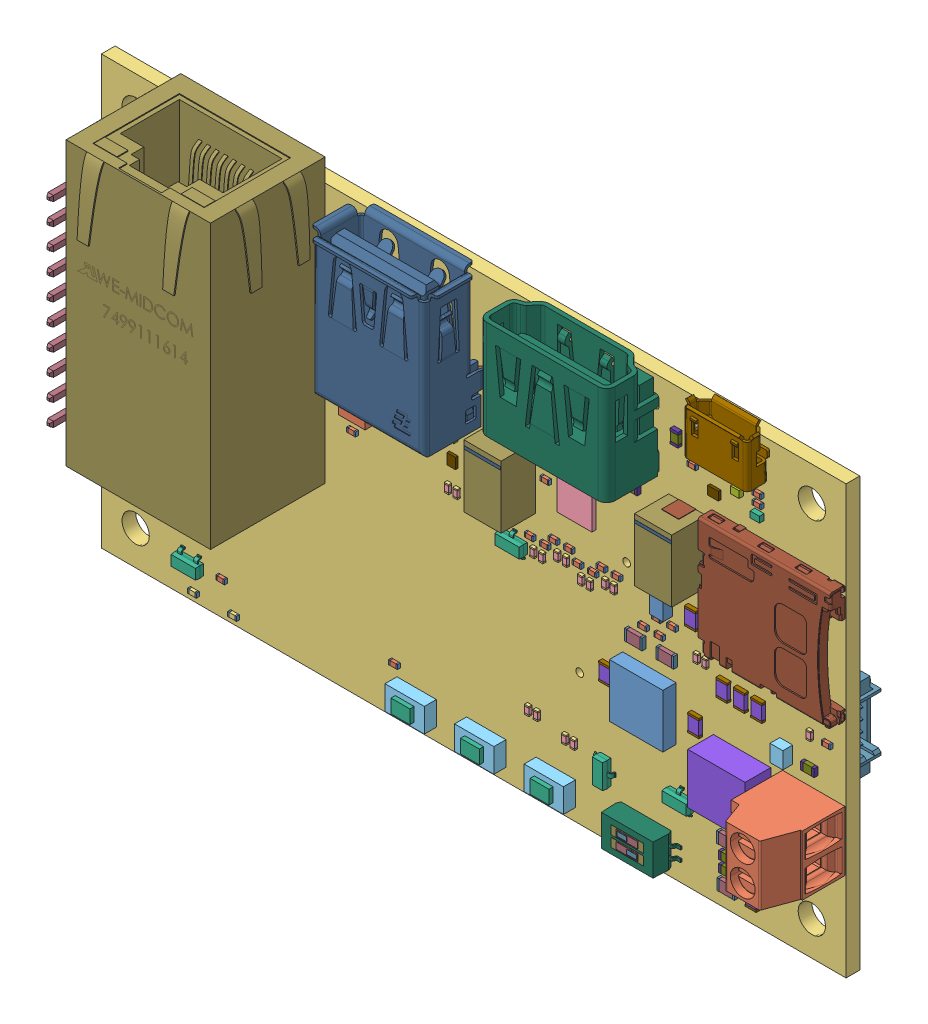
SolidWorks assembly ASG003_3D_MODEL, configuration Default. Lengths in mm. (continued)
Components (placement in the parent): (continued)
- ASG003_3D_MODEL.step-1: ASG003_3D_MODEL.step [Default] at origin size (87.04 52.68 23.65) (continued)
  - D6.step-1: D6.step [Default] at origin size (1 0.8 0.5) (continued)
    - 870940960.step-1: 870940960.step [Default] at (41.166 32.031 0) size (1 0.8 0.5) (continued)
      - Extruded-31.step-1: Extruded-31.step [Default] at origin size (1 0.8 0.5)
  - D5.step-1: D5.step [Default] at origin size (1 0.8 0.5)
    - 870940960.step-1: 870940960.step [Default] at (35.166 32.031 0) size (1 0.8 0.5)
      - Extruded-31.step-1: Extruded-31.step [Default] at origin size (1 0.8 0.5)
  - D4.step-1: D4.step [Default] at origin size (1 0.8 0.5)
    - 870940960.step-1: 870940960.step [Default] at (44.881 32.031 0) size (1 0.8 0.5)
      - Extruded-31.step-1: Extruded-31.step [Default] at origin size (1 0.8 0.5)
  - D2.step-1: D2.step [Default] at origin size (1.02 0.52 0.36)
    - 870944640.step-1: 870944640.step [Default] at (10.9212 1.0646 0) size (1.01 0.51 0.36)
      - Extruded-28.step-1: Extruded-28.step [Default] at origin size (1.01 0.51 0.36)
    - 870940480.step-1: 870940480.step [Default] at (10.4912 1.0646 0) size (0.16 0.52 0.35)
      - Extruded.step-1: Extruded.step [Default] at origin size (0.16 0.52 0.35)
    - 870940480.step-2: 870940480.step [Default] at (11.3512 1.0646 0) size (0.16 0.52 0.35)
      - Extruded.step-1: Extruded.step [Default] at origin size (0.16 0.52 0.35)
  - C57.step-1: C57.step [Default] at origin size (1.3 2.04 0.45)
    - 740904480.step-1: 740904480.step [Default] at (69.215 27.686 0) size (1.25 2 0.45)
      - Extruded-32.step-1: Extruded-32.step [Default] at origin size (1.25 2 0.45)
    - 740902240.step-1: 740902240.step [Default] at (69.215 26.7735 0) size (1.3 0.23 0.45)
      - Extruded-33.step-1: Extruded-33.step [Default] at origin size (1.3 0.23 0.45)
    - 740902240.step-2: 740902240.step [Default] at (69.215 28.586 0) size (1.3 0.23 0.45)
      - Extruded-33.step-1: Extruded-33.step [Default] at origin size (1.3 0.23 0.45)
  - C47.step-1: C47.step [Default] at origin size (1.3 2.04 0.45)
    - 740902240.step-1: 740902240.step [Default] at (72.8972 21.3736 0) size (1.3 0.23 0.45)
      - Extruded-33.step-1: Extruded-33.step [Default] at origin size (1.3 0.23 0.45)
    - 740902240.step-2: 740902240.step [Default] at (72.8972 23.1861 0) size (1.3 0.23 0.45)
      - Extruded-33.step-1: Extruded-33.step [Default] at origin size (1.3 0.23 0.45)
    - 740904480.step-1: 740904480.step [Default] at (72.8972 22.2736 0) size (1.25 2 0.45)
      - Extruded-32.step-1: Extruded-32.step [Default] at origin size (1.25 2 0.45)
  - C46.step-1: C46.step [Default] at origin size (1.3 2.04 0.45)
    - 740902240.step-1: 740902240.step [Default] at (76.9612 21.3736 0) size (1.3 0.23 0.45)
      - Extruded-33.step-1: Extruded-33.step [Default] at origin size (1.3 0.23 0.45)
    - 740902240.step-2: 740902240.step [Default] at (76.9612 23.1861 0) size (1.3 0.23 0.45)
      - Extruded-33.step-1: Extruded-33.step [Default] at origin size (1.3 0.23 0.45)
    - 740904480.step-1: 740904480.step [Default] at (76.9612 22.2736 0) size (1.25 2 0.45)
      - Extruded-32.step-1: Extruded-32.step [Default] at origin size (1.25 2 0.45)
  - C45.step-1: C45.step [Default] at origin size (1.3 2.04 0.45)
    - 740902240.step-1: 740902240.step [Default] at (74.9292 21.3736 0) size (1.3 0.23 0.45)
      - Extruded-33.step-1: Extruded-33.step [Default] at origin size (1.3 0.23 0.45)
    - 740902240.step-2: 740902240.step [Default] at (74.9292 23.1861 0) size (1.3 0.23 0.45)
      - Extruded-33.step-1: Extruded-33.step [Default] at origin size (1.3 0.23 0.45)
    - 740904480.step-1: 740904480.step [Default] at (74.9292 22.2736 0) size (1.25 2 0.45)
      - Extruded-32.step-1: Extruded-32.step [Default] at origin size (1.25 2 0.45)
  - C44.step-1: C44.step [Default] at origin size (1.02 0.52 0.36)
    - 870940480.step-1: 870940480.step [Default] at (29.084 26.6678 0) size (0.16 0.52 0.35)
      - Extruded.step-1: Extruded.step [Default] at origin size (0.16 0.52 0.35)
    - 870940480.step-2: 870940480.step [Default] at (29.944 26.6678 0) size (0.16 0.52 0.35)
      - Extruded.step-1: Extruded.step [Default] at origin size (0.16 0.52 0.35)
    - 870940640.step-1: 870940640.step [Default] at (29.514 26.6678 0) size (1.01 0.51 0.36)
      - Extruded-0.step-1: Extruded-0.step [Default] at origin size (1.01 0.51 0.36)
  - C43.step-1: C43.step [Default] at origin size (1.02 0.52 0.36)
    - 870940480.step-1: 870940480.step [Default] at (76.455 43 0) size (0.16 0.52 0.35)
      - Extruded.step-1: Extruded.step [Default] at origin size (0.16 0.52 0.35)
    - 870940480.step-2: 870940480.step [Default] at (77.315 43 0) size (0.16 0.52 0.35)
      - Extruded.step-1: Extruded.step [Default] at origin size (0.16 0.52 0.35)
    - 870940640.step-1: 870940640.step [Default] at (76.885 43 0) size (1.01 0.51 0.36)
      - Extruded-0.step-1: Extruded-0.step [Default] at origin size (1.01 0.51 0.36)
  - C42.step-1: C42.step [Default] at origin size (1.02 0.52 0.36)
    - 870940480.step-1: 870940480.step [Default] at (76.455 44.016 0) size (0.16 0.52 0.35)
      - Extruded.step-1: Extruded.step [Default] at origin size (0.16 0.52 0.35)
    - 870940480.step-2: 870940480.step [Default] at (77.315 44.016 0) size (0.16 0.52 0.35)
      - Extruded.step-1: Extruded.step [Default] at origin size (0.16 0.52 0.35)
    - 870940640.step-1: 870940640.step [Default] at (76.885 44.016 0) size (1.01 0.51 0.36)
      - Extruded-0.step-1: Extruded-0.step [Default] at origin size (1.01 0.51 0.36)
  - C41.step-1: C41.step [Default] at origin size (1.02 0.52 0.36)
    - 870940480.step-1: 870940480.step [Default] at (68.835 44.143 0) size (0.16 0.52 0.35)
      - Extruded.step-1: Extruded.step [Default] at origin size (0.16 0.52 0.35)
    - 870940480.step-2: 870940480.step [Default] at (69.695 44.143 0) size (0.16 0.52 0.35)
      - Extruded.step-1: Extruded.step [Default] at origin size (0.16 0.52 0.35)
    - 870940640.step-1: 870940640.step [Default] at (69.265 44.143 0) size (1.01 0.51 0.36)
      - Extruded-0.step-1: Extruded-0.step [Default] at origin size (1.01 0.51 0.36)
  - C40.step-1: C40.step [Default] at origin size (4.35 7.4 4.01)
    - 870941440.step-1: 870941440.step [Default] at (68.4522 37.8735 0) size (4.3 0.35 4.01)
      - Extruded-34.step-1: Extruded-34.step [Default] at origin size (4.3 0.35 4.01)
    - 870941600.step-1: 870941600.step [Default] at (68.4522 31.3736 0) size (2 0.2 2)
      - Extruded-35.step-1: Extruded-35.step [Default] at origin size (2 0.2 2)
    - 870941600.step-2: 870941600.step [Default] at (68.4522 38.5736 0) size (2 0.2 2)
      - Extruded-35.step-1: Extruded-35.step [Default] at origin size (2 0.2 2)
    - 870941760.step-1: 870941760.step [Default] at (68.4523 34.9735 0) size (4.35 7.3 4)
      - Extruded-36.step-1: Extruded-36.step [Default] at origin size (4.35 7.3 4)
  - C39.step-1: C39.step [Default] at origin size (1.02 0.52 0.36)
    - 870940480.step-1: 870940480.step [Default] at (39.673 40.1066 -1.9516) size (0.16 0.52 0.35)
      - Extruded.step-1: Extruded.step [Default] at origin size (0.16 0.52 0.35)
    - 870940480.step-2: 870940480.step [Default] at (38.813 40.1066 -1.9516) size (0.16 0.52 0.35)
      - Extruded.step-1: Extruded.step [Default] at origin size (0.16 0.52 0.35)
    - 870940640.step-1: 870940640.step [Default] at (39.243 40.1066 -1.9506) size (1.01 0.51 0.36)
      - Extruded-0.step-1: Extruded-0.step [Default] at origin size (1.01 0.51 0.36)
  - C38.step-1: C38.step [Default] at origin size (1.02 0.52 0.36)
    - 870940480.step-1: 870940480.step [Default] at (49.023 38.174 0) size (0.16 0.52 0.35)
      - Extruded.step-1: Extruded.step [Default] at origin size (0.16 0.52 0.35)
    - 870940480.step-2: 870940480.step [Default] at (49.883 38.174 0) size (0.16 0.52 0.35)
      - Extruded.step-1: Extruded.step [Default] at origin size (0.16 0.52 0.35)
    - 870940640.step-1: 870940640.step [Default] at (49.453 38.174 0) size (1.01 0.51 0.36)
      - Extruded-0.step-1: Extruded-0.step [Default] at origin size (1.01 0.51 0.36)
  - C37.step-1: C37.step [Default] at origin size (4.35 7.4 4.01)
    - 870941440.step-1: 870941440.step [Default] at (48.5132 35.3843 0) size (4.3 0.35 4.01)
      - Extruded-34.step-1: Extruded-34.step [Default] at origin size (4.3 0.35 4.01)
    - 870941600.step-1: 870941600.step [Default] at (48.5132 28.8844 0) size (2 0.2 2)
      - Extruded-35.step-1: Extruded-35.step [Default] at origin size (2 0.2 2)
    - 870941600.step-2: 870941600.step [Default] at (48.5132 36.0844 0) size (2 0.2 2)
      - Extruded-35.step-1: Extruded-35.step [Default] at origin size (2 0.2 2)
    - 870941760.step-1: 870941760.step [Default] at (48.5133 32.4843 0) size (4.35 7.3 4)
      - Extruded-36.step-1: Extruded-36.step [Default] at origin size (4.35 7.3 4)
  - C36.step-1: C36.step [Default] at origin size (0.52 1.02 0.36)
    - 870941120.step-1: 870941120.step [Default] at (41.666 26.961 0) size (0.52 0.16 0.35)
      - Extruded-1.step-1: Extruded-1.step [Default] at origin size (0.52 0.16 0.35)
    - 870941120.step-2: 870941120.step [Default] at (41.666 26.101 0) size (0.52 0.16 0.35)
      - Extruded-1.step-1: Extruded-1.step [Default] at origin size (0.52 0.16 0.35)
    - 870941280.step-1: 870941280.step [Default] at (41.666 26.531 0) size (0.51 1.01 0.36)
      - Extruded-2.step-1: Extruded-2.step [Default] at origin size (0.51 1.01 0.36)
  - C35.step-1: C35.step [Default] at origin size (0.52 1.02 0.36)
    - 870941120.step-1: 870941120.step [Default] at (40.666 26.961 0) size (0.52 0.16 0.35)
      - Extruded-1.step-1: Extruded-1.step [Default] at origin size (0.52 0.16 0.35)
    - 870941120.step-2: 870941120.step [Default] at (40.666 26.101 0) size (0.52 0.16 0.35)
      - Extruded-1.step-1: Extruded-1.step [Default] at origin size (0.52 0.16 0.35)
    - 870941280.step-1: 870941280.step [Default] at (40.666 26.531 0) size (0.51 1.01 0.36)
      - Extruded-2.step-1: Extruded-2.step [Default] at origin size (0.51 1.01 0.36)
  - C34.step-1: C34.step [Default] at origin size (1.02 0.52 0.36)
    - 870940480.step-1: 870940480.step [Default] at (83.0277 32.2771 -1.9516) size (0.16 0.52 0.35)
      - Extruded.step-1: Extruded.step [Default] at origin size (0.16 0.52 0.35)
    - 870940480.step-2: 870940480.step [Default] at (83.8877 32.2771 -1.9516) size (0.16 0.52 0.35)
      - Extruded.step-1: Extruded.step [Default] at origin size (0.16 0.52 0.35)
    - 870940640.step-1: 870940640.step [Default] at (83.4577 32.2771 -1.9506) size (1.01 0.51 0.36)
      - Extruded-0.step-1: Extruded-0.step [Default] at origin size (1.01 0.51 0.36)
  - C32.step-1: C32.step [Default] at origin size (0.52 1.02 0.36)
    - 870941120.step-1: 870941120.step [Default] at (22.148 19.554 -1.9516) size (0.52 0.16 0.35)
      - Extruded-1.step-1: Extruded-1.step [Default] at origin size (0.52 0.16 0.35)
    - 870941120.step-2: 870941120.step [Default] at (22.148 18.694 -1.9516) size (0.52 0.16 0.35)
      - Extruded-1.step-1: Extruded-1.step [Default] at origin size (0.52 0.16 0.35)
    - 870941280.step-1: 870941280.step [Default] at (22.148 19.124 -1.9506) size (0.51 1.01 0.36)
      - Extruded-2.step-1: Extruded-2.step [Default] at origin size (0.51 1.01 0.36)
  - C31.step-1: C31.step [Default] at origin size (0.52 1.02 0.36)
    - 870941120.step-1: 870941120.step [Default] at (11.607 19.554 -1.9516) size (0.52 0.16 0.35)
      - Extruded-1.step-1: Extruded-1.step [Default] at origin size (0.52 0.16 0.35)
    - 870941120.step-2: 870941120.step [Default] at (11.607 18.694 -1.9516) size (0.52 0.16 0.35)
      - Extruded-1.step-1: Extruded-1.step [Default] at origin size (0.52 0.16 0.35)
    - 870941280.step-1: 870941280.step [Default] at (11.607 19.124 -1.9506) size (0.51 1.01 0.36)
      - Extruded-2.step-1: Extruded-2.step [Default] at origin size (0.51 1.01 0.36)
  - C30.step-1: C30.step [Default] at origin size (0.52 1.02 0.36)
    - 870941120.step-1: 870941120.step [Default] at (14.147 19.623 -1.9516) size (0.52 0.16 0.35)
      - Extruded-1.step-1: Extruded-1.step [Default] at origin size (0.52 0.16 0.35)
    - 870941120.step-2: 870941120.step [Default] at (14.147 18.763 -1.9516) size (0.52 0.16 0.35)
      - Extruded-1.step-1: Extruded-1.step [Default] at origin size (0.52 0.16 0.35)
    - 870941280.step-1: 870941280.step [Default] at (14.147 19.193 -1.9506) size (0.51 1.01 0.36)
      - Extruded-2.step-1: Extruded-2.step [Default] at origin size (0.51 1.01 0.36)
  - C29.step-1: C29.step [Default] at origin size (1.02 0.52 0.36)
    - 870940480.step-1: 870940480.step [Default] at (25.528 26.617 -1.9516) size (0.16 0.52 0.35)
      - Extruded.step-1: Extruded.step [Default] at origin size (0.16 0.52 0.35)
    - 870940480.step-2: 870940480.step [Default] at (26.388 26.617 -1.9516) size (0.16 0.52 0.35)
      - Extruded.step-1: Extruded.step [Default] at origin size (0.16 0.52 0.35)
    - 870940640.step-1: 870940640.step [Default] at (25.958 26.617 -1.9506) size (1.01 0.51 0.36)
      - Extruded-0.step-1: Extruded-0.step [Default] at origin size (1.01 0.51 0.36)
  - C28.step-1: C28.step [Default] at origin size (1.02 0.52 0.36)
    - 870940480.step-1: 870940480.step [Default] at (25.782 24.077 -1.9516) size (0.16 0.52 0.35)
      - Extruded.step-1: Extruded.step [Default] at origin size (0.16 0.52 0.35)
    - 870940480.step-2: 870940480.step [Default] at (26.642 24.077 -1.9516) size (0.16 0.52 0.35)
      - Extruded.step-1: Extruded.step [Default] at origin size (0.16 0.52 0.35)
    - 870940640.step-1: 870940640.step [Default] at (26.212 24.077 -1.9506) size (1.01 0.51 0.36)
      - Extruded-0.step-1: Extruded-0.step [Default] at origin size (1.01 0.51 0.36)
  - C27.step-1: C27.step [Default] at origin size (1.02 0.52 0.36)
    - 870940480.step-1: 870940480.step [Default] at (10.0685 26.617 -1.9516) size (0.16 0.52 0.35)
      - Extruded.step-1: Extruded.step [Default] at origin size (0.16 0.52 0.35)
    - 870940480.step-2: 870940480.step [Default] at (9.2085 26.617 -1.9516) size (0.16 0.52 0.35)
      - Extruded.step-1: Extruded.step [Default] at origin size (0.16 0.52 0.35)
    - 870940640.step-1: 870940640.step [Default] at (9.6385 26.617 -1.9506) size (1.01 0.51 0.36)
      - Extruded-0.step-1: Extruded-0.step [Default] at origin size (1.01 0.51 0.36)
  - C26.step-1: C26.step [Default] at origin size (1.02 0.52 0.36)
    - 870940480.step-1: 870940480.step [Default] at (9.878 24.077 -1.9516) size (0.16 0.52 0.35)
      - Extruded.step-1: Extruded.step [Default] at origin size (0.16 0.52 0.35)
    - 870940480.step-2: 870940480.step [Default] at (9.018 24.077 -1.9516) size (0.16 0.52 0.35)
      - Extruded.step-1: Extruded.step [Default] at origin size (0.16 0.52 0.35)
    - 870940640.step-1: 870940640.step [Default] at (9.448 24.077 -1.9506) size (1.01 0.51 0.36)
      - Extruded-0.step-1: Extruded-0.step [Default] at origin size (1.01 0.51 0.36)
  - C25.step-1: C25.step [Default] at origin size (1.02 0.52 0.36)
    - 870940480.step-1: 870940480.step [Default] at (7.923 33.147 -1.9516) size (0.16 0.52 0.35)
      - Extruded.step-1: Extruded.step [Default] at origin size (0.16 0.52 0.35)
    - 870940480.step-2: 870940480.step [Default] at (7.063 33.147 -1.9516) size (0.16 0.52 0.35)
      - Extruded.step-1: Extruded.step [Default] at origin size (0.16 0.52 0.35)
    - 870940640.step-1: 870940640.step [Default] at (7.493 33.147 -1.9506) size (1.01 0.51 0.36)
      - Extruded-0.step-1: Extruded-0.step [Default] at origin size (1.01 0.51 0.36)
  - C24.step-1: C24.step [Default] at origin size (1.02 0.52 0.36)
    - 870940480.step-1: 870940480.step [Default] at (9.603 33.147 -1.9516) size (0.16 0.52 0.35)
      - Extruded.step-1: Extruded.step [Default] at origin size (0.16 0.52 0.35)
    - 870940480.step-2: 870940480.step [Default] at (10.463 33.147 -1.9516) size (0.16 0.52 0.35)
      - Extruded.step-1: Extruded.step [Default] at origin size (0.16 0.52 0.35)
    - 870940640.step-1: 870940640.step [Default] at (10.033 33.147 -1.9506) size (1.01 0.51 0.36)
      - Extruded-0.step-1: Extruded-0.step [Default] at origin size (1.01 0.51 0.36)
  - C23.step-1: C23.step [Default] at origin size (1.3 2.04 0.45)
    - 740904480.step-1: 740904480.step [Default] at (78.486 26.162 -2.0506) size (1.25 2 0.45)
      - Extruded-32.step-1: Extruded-32.step [Default] at origin size (1.25 2 0.45)
    - 740902240.step-1: 740902240.step [Default] at (78.486 27.0745 -2.0516) size (1.3 0.23 0.45)
      - Extruded-33.step-1: Extruded-33.step [Default] at origin size (1.3 0.23 0.45)
    - 740902240.step-2: 740902240.step [Default] at (78.486 25.262 -2.0516) size (1.3 0.23 0.45)
      - Extruded-33.step-1: Extruded-33.step [Default] at origin size (1.3 0.23 0.45)
  - C22.step-1: C22.step [Default] at origin size (0.52 1.02 0.36)
    - 870941120.step-1: 870941120.step [Default] at (7.493 41.099 -1.9516) size (0.52 0.16 0.35)
      - Extruded-1.step-1: Extruded-1.step [Default] at origin size (0.52 0.16 0.35)
    - 870941120.step-2: 870941120.step [Default] at (7.493 41.959 -1.9516) size (0.52 0.16 0.35)
      - Extruded-1.step-1: Extruded-1.step [Default] at origin size (0.52 0.16 0.35)
    - 870941280.step-1: 870941280.step [Default] at (7.493 41.529 -1.9506) size (0.51 1.01 0.36)
      - Extruded-2.step-1: Extruded-2.step [Default] at origin size (0.51 1.01 0.36)
  - C21.step-1: C21.step [Default] at origin size (0.52 1.02 0.36)
    - 870941120.step-1: 870941120.step [Default] at (8.636 41.099 -1.9516) size (0.52 0.16 0.35)
      - Extruded-1.step-1: Extruded-1.step [Default] at origin size (0.52 0.16 0.35)
    - 870941120.step-2: 870941120.step [Default] at (8.636 41.959 -1.9516) size (0.52 0.16 0.35)
      - Extruded-1.step-1: Extruded-1.step [Default] at origin size (0.52 0.16 0.35)
    - 870941280.step-1: 870941280.step [Default] at (8.636 41.529 -1.9506) size (0.51 1.01 0.36)
      - Extruded-2.step-1: Extruded-2.step [Default] at origin size (0.51 1.01 0.36)
  - C19.step-1: C19.step [Default] at origin size (1.6 0.9 0.46)
    - 870942080.step-1: 870942080.step [Default] at (62.892 37.465 0) size (0.3 0.9 0.46)
      - Extruded-13.step-1: Extruded-13.step [Default] at origin size (0.3 0.9 0.46)
    - 870942080.step-2: 870942080.step [Default] at (61.592 37.465 0) size (0.3 0.9 0.46)
      - Extruded-13.step-1: Extruded-13.step [Default] at origin size (0.3 0.9 0.46)
    - 870942240.step-1: 870942240.step [Default] at (62.242 37.465 0) size (1 0.9 0.45)
      - Extruded-12.step-1: Extruded-12.step [Default] at origin size (1 0.9 0.45)
  - C18.step-1: C18.step [Default] at origin size (1.02 0.52 0.36)
    - 870940480.step-1: 870940480.step [Default] at (53.722 33.3988 -1.9516) size (0.16 0.52 0.35)
      - Extruded.step-1: Extruded.step [Default] at origin size (0.16 0.52 0.35)
    - 870940480.step-2: 870940480.step [Default] at (54.582 33.3988 -1.9516) size (0.16 0.52 0.35)
      - Extruded.step-1: Extruded.step [Default] at origin size (0.16 0.52 0.35)
    - 870940640.step-1: 870940640.step [Default] at (54.152 33.3988 -1.9506) size (1.01 0.51 0.36)
      - Extruded-0.step-1: Extruded-0.step [Default] at origin size (1.01 0.51 0.36)
  - C17.step-1: C17.step [Default] at origin size (1.02 0.52 0.36)
    - 870940480.step-1: 870940480.step [Default] at (57.7824 32.2304 -1.9516) size (0.16 0.52 0.35)
      - Extruded.step-1: Extruded.step [Default] at origin size (0.16 0.52 0.35)
    - 870940480.step-2: 870940480.step [Default] at (56.9224 32.2304 -1.9516) size (0.16 0.52 0.35)
      - Extruded.step-1: Extruded.step [Default] at origin size (0.16 0.52 0.35)
    - 870940640.step-1: 870940640.step [Default] at (57.3524 32.2304 -1.9506) size (1.01 0.51 0.36)
      - Extruded-0.step-1: Extruded-0.step [Default] at origin size (1.01 0.51 0.36)
  - C16.step-1: C16.step [Default] at origin size (1.02 0.52 0.36)
    - 870940480.step-1: 870940480.step [Default] at (54.582 34.6434 -1.9516) size (0.16 0.52 0.35)
      - Extruded.step-1: Extruded.step [Default] at origin size (0.16 0.52 0.35)
    - 870940480.step-2: 870940480.step [Default] at (53.722 34.6434 -1.9516) size (0.16 0.52 0.35)
      - Extruded.step-1: Extruded.step [Default] at origin size (0.16 0.52 0.35)
    - 870940640.step-1: 870940640.step [Default] at (54.152 34.6434 -1.9506) size (1.01 0.51 0.36)
      - Extruded-0.step-1: Extruded-0.step [Default] at origin size (1.01 0.51 0.36)
  - C15.step-1: C15.step [Default] at origin size (0.52 1.02 0.36)
    - 870941120.step-1: 870941120.step [Default] at (51.6628 25.4722 0) size (0.52 0.16 0.35)
      - Extruded-1.step-1: Extruded-1.step [Default] at origin size (0.52 0.16 0.35)
    - 870941120.step-2: 870941120.step [Default] at (51.6628 24.6122 0) size (0.52 0.16 0.35)
      - Extruded-1.step-1: Extruded-1.step [Default] at origin size (0.52 0.16 0.35)
    - 870941280.step-1: 870941280.step [Default] at (51.6628 25.0422 0) size (0.51 1.01 0.36)
      - Extruded-2.step-1: Extruded-2.step [Default] at origin size (0.51 1.01 0.36)
  - C14.step-1: C14.step [Default] at origin size (0.52 1.02 0.36)
    - 870941120.step-1: 870941120.step [Default] at (50.6468 25.4722 0) size (0.52 0.16 0.35)
      - Extruded-1.step-1: Extruded-1.step [Default] at origin size (0.52 0.16 0.35)
    - 870941120.step-2: 870941120.step [Default] at (50.6468 24.6122 0) size (0.52 0.16 0.35)
      - Extruded-1.step-1: Extruded-1.step [Default] at origin size (0.52 0.16 0.35)
    - 870941280.step-1: 870941280.step [Default] at (50.6468 25.0422 0) size (0.51 1.01 0.36)
      - Extruded-2.step-1: Extruded-2.step [Default] at origin size (0.51 1.01 0.36)
  - C13.step-1: C13.step [Default] at origin size (0.52 1.02 0.36)
    - 870941120.step-1: 870941120.step [Default] at (54.4568 26.4882 0) size (0.52 0.16 0.35)
      - Extruded-1.step-1: Extruded-1.step [Default] at origin size (0.52 0.16 0.35)
    - 870941120.step-2: 870941120.step [Default] at (54.4568 25.6282 0) size (0.52 0.16 0.35)
      - Extruded-1.step-1: Extruded-1.step [Default] at origin size (0.52 0.16 0.35)
    - 870941280.step-1: 870941280.step [Default] at (54.4568 26.0582 0) size (0.51 1.01 0.36)
      - Extruded-2.step-1: Extruded-2.step [Default] at origin size (0.51 1.01 0.36)
  - C12.step-1: C12.step [Default] at origin size (0.52 1.02 0.36)
    - 870941120.step-1: 870941120.step [Default] at (53.4408 26.4882 0) size (0.52 0.16 0.35)
      - Extruded-1.step-1: Extruded-1.step [Default] at origin size (0.52 0.16 0.35)
    - 870941120.step-2: 870941120.step [Default] at (53.4408 25.6282 0) size (0.52 0.16 0.35)
      - Extruded-1.step-1: Extruded-1.step [Default] at origin size (0.52 0.16 0.35)
    - 870941280.step-1: 870941280.step [Default] at (53.4408 26.0582 0) size (0.51 1.01 0.36)
      - Extruded-2.step-1: Extruded-2.step [Default] at origin size (0.51 1.01 0.36)
  - C11.step-1: C11.step [Default] at origin size (0.52 1.02 0.36)
    - 870941120.step-1: 870941120.step [Default] at (57.2508 25.4722 0) size (0.52 0.16 0.35)
      - Extruded-1.step-1: Extruded-1.step [Default] at origin size (0.52 0.16 0.35)
    - 870941120.step-2: 870941120.step [Default] at (57.2508 24.6122 0) size (0.52 0.16 0.35)
      - Extruded-1.step-1: Extruded-1.step [Default] at origin size (0.52 0.16 0.35)
    - 870941280.step-1: 870941280.step [Default] at (57.2508 25.0422 0) size (0.51 1.01 0.36)
      - Extruded-2.step-1: Extruded-2.step [Default] at origin size (0.51 1.01 0.36)
  - C10.step-1: C10.step [Default] at origin size (0.52 1.02 0.36)
    - 870941120.step-1: 870941120.step [Default] at (56.2348 25.4722 0) size (0.52 0.16 0.35)
      - Extruded-1.step-1: Extruded-1.step [Default] at origin size (0.52 0.16 0.35)
    - 870941120.step-2: 870941120.step [Default] at (56.2348 24.6122 0) size (0.52 0.16 0.35)
      - Extruded-1.step-1: Extruded-1.step [Default] at origin size (0.52 0.16 0.35)
    - 870941280.step-1: 870941280.step [Default] at (56.2348 25.0422 0) size (0.51 1.01 0.36)
      - Extruded-2.step-1: Extruded-2.step [Default] at origin size (0.51 1.01 0.36)
  - C9.step-1: C9.step [Default] at origin size (0.52 1.02 0.36)
    - 870941120.step-1: 870941120.step [Default] at (60.0448 26.4882 0) size (0.52 0.16 0.35)
      - Extruded-1.step-1: Extruded-1.step [Default] at origin size (0.52 0.16 0.35)
    - 870941120.step-2: 870941120.step [Default] at (60.0448 25.6282 0) size (0.52 0.16 0.35)
      - Extruded-1.step-1: Extruded-1.step [Default] at origin size (0.52 0.16 0.35)
    - 870941280.step-1: 870941280.step [Default] at (60.0448 26.0582 0) size (0.51 1.01 0.36)
      - Extruded-2.step-1: Extruded-2.step [Default] at origin size (0.51 1.01 0.36)
  - C8.step-1: C8.step [Default] at origin size (0.52 1.02 0.36)
    - 870941120.step-1: 870941120.step [Default] at (59.0288 26.4882 0) size (0.52 0.16 0.35)
      - Extruded-1.step-1: Extruded-1.step [Default] at origin size (0.52 0.16 0.35)
    - 870941120.step-2: 870941120.step [Default] at (59.0288 25.6282 0) size (0.52 0.16 0.35)
      - Extruded-1.step-1: Extruded-1.step [Default] at origin size (0.52 0.16 0.35)
    - 870941280.step-1: 870941280.step [Default] at (59.0288 26.0582 0) size (0.51 1.01 0.36)
      - Extruded-2.step-1: Extruded-2.step [Default] at origin size (0.51 1.01 0.36)
  - C6.step-1: C6.step [Default] at origin size (1.6 0.9 0.46)
    - 870942080.step-1: 870942080.step [Default] at (72.7044 4.138 0) size (0.3 0.9 0.46)
      - Extruded-13.step-1: Extruded-13.step [Default] at origin size (0.3 0.9 0.46)
    - 870942080.step-2: 870942080.step [Default] at (74.0044 4.138 0) size (0.3 0.9 0.46)
      - Extruded-13.step-1: Extruded-13.step [Default] at origin size (0.3 0.9 0.46)
    - 870942240.step-1: 870942240.step [Default] at (73.3544 4.138 0) size (1 0.9 0.45)
      - Extruded-12.step-1: Extruded-12.step [Default] at origin size (1 0.9 0.45)
  - C5.step-1: C5.step [Default] at origin size (1.6 0.9 0.46)
    - 870942080.step-1: 870942080.step [Default] at (72.7044 5.4842 0) size (0.3 0.9 0.46)
      - Extruded-13.step-1: Extruded-13.step [Default] at origin size (0.3 0.9 0.46)
    - 870942080.step-2: 870942080.step [Default] at (74.0044 5.4842 0) size (0.3 0.9 0.46)
      - Extruded-13.step-1: Extruded-13.step [Default] at origin size (0.3 0.9 0.46)
    - 870942240.step-1: 870942240.step [Default] at (73.3544 5.4842 0) size (1 0.9 0.45)
      - Extruded-12.step-1: Extruded-12.step [Default] at origin size (1 0.9 0.45)
  - C4.step-1: C4.step [Default] at origin size (2.04 1.3 0.45)
    - 870943200.step-1: 870943200.step [Default] at (77.139 5.5604 0) size (2 1.25 0.45)
      - Extruded-37.step-1: Extruded-37.step [Default] at origin size (2 1.25 0.45)
    - 870943360.step-1: 870943360.step [Default] at (78.0515 5.5604 0) size (0.23 1.3 0.45)
      - Extruded-38.step-1: Extruded-38.step [Default] at origin size (0.23 1.3 0.45)
    - 870943360.step-2: 870943360.step [Default] at (76.239 5.5604 0) size (0.23 1.3 0.45)
      - Extruded-38.step-1: Extruded-38.step [Default] at origin size (0.23 1.3 0.45)
  - C3.step-1: C3.step [Default] at origin size (1.3 2.04 0.45)
    - 740904480.step-1: 740904480.step [Default] at (76.3008 2.8426 0) size (1.25 2 0.45)
      - Extruded-32.step-1: Extruded-32.step [Default] at origin size (1.25 2 0.45)
    - 740902240.step-1: 740902240.step [Default] at (76.3008 1.9301 0) size (1.3 0.23 0.45)
      - Extruded-33.step-1: Extruded-33.step [Default] at origin size (1.3 0.23 0.45)
    - 740902240.step-2: 740902240.step [Default] at (76.3008 3.7426 0) size (1.3 0.23 0.45)
      - Extruded-33.step-1: Extruded-33.step [Default] at origin size (1.3 0.23 0.45)
  - C2.step-1: C2.step [Default] at origin size (2.04 1.3 0.45)
    - 870943200.step-1: 870943200.step [Default] at (73.3798 2.4108 0) size (2 1.25 0.45)
      - Extruded-37.step-1: Extruded-37.step [Default] at origin size (2 1.25 0.45)
    - 870943360.step-1: 870943360.step [Default] at (72.4673 2.4108 0) size (0.23 1.3 0.45)
      - Extruded-38.step-1: Extruded-38.step [Default] at origin size (0.23 1.3 0.45)
    - 870943360.step-2: 870943360.step [Default] at (74.2798 2.4108 0) size (0.23 1.3 0.45)
      - Extruded-38.step-1: Extruded-38.step [Default] at origin size (0.23 1.3 0.45)
  - C1.step-1: C1.step [Default] at origin size (2.04 1.3 0.45)
    - 870943200.step-1: 870943200.step [Default] at (73.3544 7.1606 0) size (2 1.25 0.45)
      - Extruded-37.step-1: Extruded-37.step [Default] at origin size (2 1.25 0.45)
    - 870943360.step-1: 870943360.step [Default] at (72.4419 7.1606 0) size (0.23 1.3 0.45)
      - Extruded-38.step-1: Extruded-38.step [Default] at origin size (0.23 1.3 0.45)
    - 870943360.step-2: 870943360.step [Default] at (74.2544 7.1606 0) size (0.23 1.3 0.45)
      - Extruded-38.step-1: Extruded-38.step [Default] at origin size (0.23 1.3 0.45)
  - P1.step-1: P1.step [Default] at origin size (69.37 12.14 8.38)
    - SEAM-50-03.5-S-08-2-A-K-TR.step-1: SEAM-50-03.5-S-08-2-A-K-TR.step [Default] at (43.4999 7.4255 -4.9661) x (1 0 0) z (0 1 0) size (69.37 8.38 12.14)
      - _SEAM-50-03.5-L-08-1-A-K-TR_body.step-1: _SEAM-50-03.5-L-08-1-A-K-TR_body.step [Default] at origin size (69.37 8.38 12.14)
      - _SEAM-50-03.5-L-08-1-A-K-TR_conn.step-1: _SEAM-50-03.5-L-08-1-A-K-TR_conn.step [Default] at origin size (67.97 5.75 11.63)
      - _SEAM_K_Pad_08.step-1: _SEAM_K_Pad_08.step [Default] at (0 2.7432 0) size (8.26 0.13 8.26)
      - _SEAM_Triangle.step-1: _SEAM_Triangle.step [Default] at (32.2834 1.3462 -4.2164) x (-1 0 0) z (0 0 -1) size (1.02 1.27 0.13)
  - C51.step-1: C51.step [Default] at origin size (2.04 1.3 0.45)
    - 870943360.step-1: 870943360.step [Default] at (63.4848 22.2482 0) size (0.23 1.3 0.45)
      - Extruded-38.step-1: Extruded-38.step [Default] at origin size (0.23 1.3 0.45)
    - 870943360.step-2: 870943360.step [Default] at (61.6723 22.2482 0) size (0.23 1.3 0.45)
      - Extruded-38.step-1: Extruded-38.step [Default] at origin size (0.23 1.3 0.45)
    - 870943200.step-1: 870943200.step [Default] at (62.5848 22.2482 0) size (2 1.25 0.45)
      - Extruded-37.step-1: Extruded-37.step [Default] at origin size (2 1.25 0.45)
  - C52.step-1: C52.step [Default] at origin size (1.3 2.04 0.45)
    - 740902240.step-1: 740902240.step [Default] at (69.5952 17.9666 0) size (1.3 0.23 0.45)
      - Extruded-33.step-1: Extruded-33.step [Default] at origin size (1.3 0.23 0.45)
    - 740902240.step-2: 740902240.step [Default] at (69.5952 16.1541 0) size (1.3 0.23 0.45)
      - Extruded-33.step-1: Extruded-33.step [Default] at origin size (1.3 0.23 0.45)
    - 740904480.step-1: 740904480.step [Default] at (69.5952 17.0666 0) size (1.25 2 0.45)
      - Extruded-32.step-1: Extruded-32.step [Default] at origin size (1.25 2 0.45)
  - C53.step-1: C53.step [Default] at origin size (1.3 2.04 0.45)
    - 740902240.step-1: 740902240.step [Default] at (59.1812 17.9666 0) size (1.3 0.23 0.45)
      - Extruded-33.step-1: Extruded-33.step [Default] at origin size (1.3 0.23 0.45)
    - 740902240.step-2: 740902240.step [Default] at (59.1812 16.1541 0) size (1.3 0.23 0.45)
      - Extruded-33.step-1: Extruded-33.step [Default] at origin size (1.3 0.23 0.45)
    - 740904480.step-1: 740904480.step [Default] at (59.1812 17.0666 0) size (1.25 2 0.45)
      - Extruded-32.step-1: Extruded-32.step [Default] at origin size (1.25 2 0.45)
  - C54.step-1: C54.step [Default] at origin size (2.04 1.3 0.45)
    - 870943360.step-1: 870943360.step [Default] at (65.3678 22.2482 0) size (0.23 1.3 0.45)
      - Extruded-38.step-1: Extruded-38.step [Default] at origin size (0.23 1.3 0.45)
    - 870943360.step-2: 870943360.step [Default] at (67.1803 22.2482 0) size (0.23 1.3 0.45)
      - Extruded-38.step-1: Extruded-38.step [Default] at origin size (0.23 1.3 0.45)
    - 870943200.step-1: 870943200.step [Default] at (66.2678 22.2482 0) size (2 1.25 0.45)
      - Extruded-37.step-1: Extruded-37.step [Default] at origin size (2 1.25 0.45)
  - C55.step-1: C55.step [Default] at origin size (1.02 0.52 0.36)
    - 870940640.step-1: 870940640.step [Default] at (61.3982 17.1936 -1.9506) size (1.01 0.51 0.36)
      - Extruded-0.step-1: Extruded-0.step [Default] at origin size (1.01 0.51 0.36)
    - 870940480.step-1: 870940480.step [Default] at (60.9682 17.1936 -1.9516) size (0.16 0.52 0.35)
      - Extruded.step-1: Extruded.step [Default] at origin size (0.16 0.52 0.35)
    - 870940480.step-2: 870940480.step [Default] at (61.8282 17.1936 -1.9516) size (0.16 0.52 0.35)
      - Extruded.step-1: Extruded.step [Default] at origin size (0.16 0.52 0.35)
  - C56.step-1: C56.step [Default] at origin size (1.02 0.52 0.36)
    - 870940640.step-1: 870940640.step [Default] at (67.6648 17.219 -1.9506) size (1.01 0.51 0.36)
      - Extruded-0.step-1: Extruded-0.step [Default] at origin size (1.01 0.51 0.36)
    - 870940480.step-1: 870940480.step [Default] at (68.0948 17.219 -1.9516) size (0.16 0.52 0.35)
      - Extruded.step-1: Extruded.step [Default] at origin size (0.16 0.52 0.35)
    - 870940480.step-2: 870940480.step [Default] at (67.2348 17.219 -1.9516) size (0.16 0.52 0.35)
      - Extruded.step-1: Extruded.step [Default] at origin size (0.16 0.52 0.35)
  - R41.step-1: R41.step [Default] at origin size (1.02 0.52 0.36)
    - 870940640.step-1: 870940640.step [Default] at (67.6648 15.9744 -1.9506) size (1.01 0.51 0.36)
      - Extruded-0.step-1: Extruded-0.step [Default] at origin size (1.01 0.51 0.36)
    - 870940480.step-1: 870940480.step [Default] at (67.2348 15.9744 -1.9516) size (0.16 0.52 0.35)
      - Extruded.step-1: Extruded.step [Default] at origin size (0.16 0.52 0.35)
    - 870940480.step-2: 870940480.step [Default] at (68.0948 15.9744 -1.9516) size (0.16 0.52 0.35)
      - Extruded.step-1: Extruded.step [Default] at origin size (0.16 0.52 0.35)
  - R42.step-1: R42.step [Default] at origin size (1.02 0.52 0.36)
    - 870940640.step-1: 870940640.step [Default] at (61.3982 15.9236 -1.9506) size (1.01 0.51 0.36)
      - Extruded-0.step-1: Extruded-0.step [Default] at origin size (1.01 0.51 0.36)
    - 870940480.step-1: 870940480.step [Default] at (61.8282 15.9236 -1.9516) size (0.16 0.52 0.35)
      - Extruded.step-1: Extruded.step [Default] at origin size (0.16 0.52 0.35)
    - 870940480.step-2: 870940480.step [Default] at (60.9682 15.9236 -1.9516) size (0.16 0.52 0.35)
      - Extruded.step-1: Extruded.step [Default] at origin size (0.16 0.52 0.35)
  - R43.step-1: R43.step [Default] at origin size (0.52 1.02 0.36)
    - 870941280.step-1: 870941280.step [Default] at (64.3882 15.4736 -1.9506) size (0.51 1.01 0.36)
      - Extruded-2.step-1: Extruded-2.step [Default] at origin size (0.51 1.01 0.36)
    - 870941120.step-1: 870941120.step [Default] at (64.3882 15.9036 -1.9516) size (0.52 0.16 0.35)
      - Extruded-1.step-1: Extruded-1.step [Default] at origin size (0.52 0.16 0.35)
    - 870941120.step-2: 870941120.step [Default] at (64.3882 15.0436 -1.9516) size (0.52 0.16 0.35)
      - Extruded-1.step-1: Extruded-1.step [Default] at origin size (0.52 0.16 0.35)
  - U6.step-1: U6.step [Default] at origin size (6.25 6.25 1.55)
    - 870945760.step-1: 870945760.step [Default] at (64.3882 17.1936 0.37) size (6.25 6.25 1.55)
      - Extruded-39.step-1: Extruded-39.step [Default] at origin size (6.25 6.25 1.55)
  - Q7.step-1: Q7.step [Default] at origin size (2.9 2.42 1)
    - SW3dPS-SOT-23.step-1: SW3dPS-SOT-23.step [Default] at (67.8839 8.593 0.498) x (0 -1 0) z (-1 0 0) size (2.42 1 2.9)
  - P9.step-1: P9.step [Default] at origin size (7.3 7 12)
    - c-1546551-2-a-3d_RGB52224.step-1: c-1546551-2-a-3d_RGB52224.step [Default] at (86.8889 13.8152 2.4127) x (0 1 0) z (1 0 0) size (7 12 7.3)
  - Board.step-1: Board.step [Default] at (0 0 -1.6006) size (87 50 1.6)
